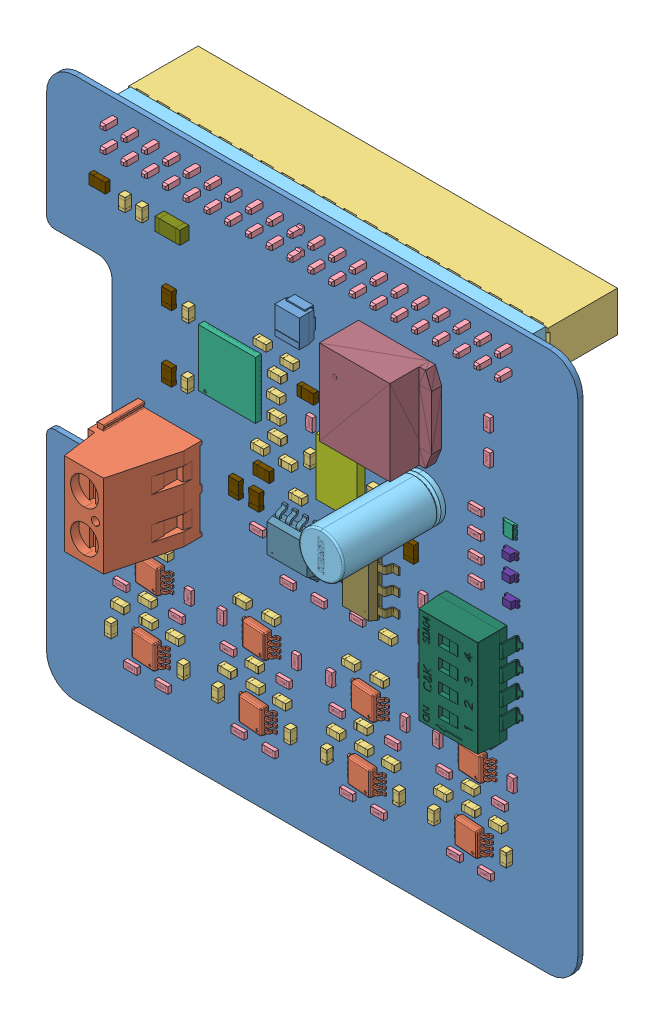
SolidWorks assembly Top, configuration Default. Lengths in mm.
Overall size (64.99 66.2 32.51).
275 component instances, 24 part files, 0 mates.
Components (placement in the parent):
- Top.step-1: Top.step [Default] at origin size (64.99 66.2 32.51)
  - Board.step-1: Board.step [Default] at origin size (64.99 66.2 0.62)
    - Open CASCADE STEP translator 6.8 4.1.1.step-1: Open CASCADE STEP translator 6.8 4.1.1.step [Default] at (0 0 -0.6237) size (64.99 66.2 0.62)
  - U5_amplification3.step-1: U5_amplification3.step [Default] at origin size (4.97 3 1.44)
    - OPA2376AIDGKR--3DModel-STEP-56544.step-1: OPA2376AIDGKR--3DModel-STEP-56544.step [Default] at (49.5292 44.6395 0.3749) x (0 1 0) z (0.997519 0 0.070401) size (3 1.1 4.9)
  - C1_PreAmp3.step-1: C1_PreAmp3.step [Default] at origin size (0.8 1.6 0.8)
    - C0603.step-1: C0603.step [Default] at (53.5531 36.5001 0.4127) x (0 -1 0) z (0 0 1) size (1.6 0.8 0.8)
  - C2_PreAmp3.step-1: C2_PreAmp3.step [Default] at origin size (1.6 0.8 0.8)
    - C0603.step-1: C0603.step [Default] at (45.8499 39.4031 0.4127) x (1 0 0) z (0 0 1) size (1.6 0.8 0.8)
  - C3_PreAmp3.step-1: C3_PreAmp3.step [Default] at origin size (1.6 0.8 0.8)
    - C0603.step-1: C0603.step [Default] at (49.3001 39.4481 0.4127) x (-1 0 0) z (0 0 1) size (1.6 0.8 0.8)
  - C5_PreAmp3.step-1: C5_PreAmp3.step [Default] at origin size (1.6 0.8 0.8)
    - C0603.step-1: C0603.step [Default] at (52.5544 39.4034 0.4127) x (-1 0 0) z (0 0 1) size (1.6 0.8 0.8)
  - C6_PreAmp3.step-1: C6_PreAmp3.step [Default] at origin size (0.8 1.6 0.8)
    - C0603.step-1: C0603.step [Default] at (44.6946 36.5001 0.4127) x (0 -1 0) z (0 0 1) size (1.6 0.8 0.8)
  - C52_amplification3.step-1: C52_amplification3.step [Default] at origin size (1.6 0.8 0.8)
    - C0603.step-1: C0603.step [Default] at (49.2044 41.6576 0.4127) x (-1 0 0) z (0 0 1) size (1.6 0.8 0.8)
  - C54_amplification3.step-1: C54_amplification3.step [Default] at origin size (1.6 0.8 0.8)
    - C0603.step-1: C0603.step [Default] at (47.7041 47.6574 0.4127) x (1 0 0) z (0 0 1) size (1.6 0.8 0.8)
  - C56_amplification3.step-1: C56_amplification3.step [Default] at origin size (1.6 0.8 0.8)
    - C0603.step-1: C0603.step [Default] at (51.2044 47.6576 0.4127) x (-1 0 0) z (0 0 1) size (1.6 0.8 0.8)
  - R1_PreAmp3.step-1: R1_PreAmp3.step [Default] at origin size (0.8 1.6 0.45)
    - R0603.step-1: R0603.step [Default] at (53.5001 36.5001 -0.8615) x (1 0 0) z (0 1 0) size (0.8 0.45 1.6)
  - R2_PreAmp3.step-1: R2_PreAmp3.step [Default] at origin size (1.6 0.8 0.45)
    - R0603.step-1: R0603.step [Default] at (50.9001 33.3448 0.2378) x (0 1 0) z (1 0 0) size (0.8 0.45 1.6)
  - R3_PreAmp3.step-1: R3_PreAmp3.step [Default] at origin size (1.6 0.8 0.45)
    - R0603.step-1: R0603.step [Default] at (47.0999 33.4447 0.2378) x (0 -1 0) z (-1 0 0) size (0.8 0.45 1.6)
  - R4_PreAmp3.step-1: R4_PreAmp3.step [Default] at origin size (0.8 1.6 0.45)
    - R0603.step-1: R0603.step [Default] at (44.6554 36.5044 -0.8615) x (1 0 0) z (0 1 0) size (0.8 0.45 1.6)
  - R23_amplification3.step-1: R23_amplification3.step [Default] at origin size (0.8 1.6 0.45)
    - R0603.step-1: R0603.step [Default] at (54.1042 44.4619 0.2378) x (-1 0 0) z (0 1 0) size (0.8 0.45 1.6)
  - R26_amplification3.step-1: R26_amplification3.step [Default] at origin size (1.6 0.8 0.45)
    - R0603.step-1: R0603.step [Default] at (52.6041 41.5574 0.2378) x (0 -1 0) z (-1 0 0) size (0.8 0.45 1.6)
  - R28_amplification3.step-1: R28_amplification3.step [Default] at origin size (1.6 0.8 0.45)
    - R0603.step-1: R0603.step [Default] at (45.8044 41.5576 0.2378) x (0 1 0) z (1 0 0) size (0.8 0.45 1.6)
  - R38_amplification3.step-1: R38_amplification3.step [Default] at origin size (0.8 1.6 0.45)
    - R0603.step-1: R0603.step [Default] at (44.9999 44.6576 0.2378) x (-1 0 0) z (0 1 0) size (0.8 0.45 1.6)
  - U1_PreAmp3.step-1: U1_PreAmp3.step [Default] at origin size (4.97 3 1.44)
    - OPA2376AIDGKR--3DModel-STEP-56544.step-1: OPA2376AIDGKR--3DModel-STEP-56544.step [Default] at (49.1239 36.474 0.3749) x (0 1 0) z (0.997519 0 0.070401) size (3 1.1 4.9)
  - U5_amplification2.step-1: U5_amplification2.step [Default] at origin size (4.97 3 1.44)
    - OPA2376AIDGKR--3DModel-STEP-56544.step-1: OPA2376AIDGKR--3DModel-STEP-56544.step [Default] at (36.2292 44.5395 0.3749) x (0 1 0) z (0.997519 0 0.070401) size (3 1.1 4.9)
  - C1_PreAmp2.step-1: C1_PreAmp2.step [Default] at origin size (0.8 1.6 0.8)
    - C0603.step-1: C0603.step [Default] at (40.2531 36.4001 0.4127) x (0 -1 0) z (0 0 1) size (1.6 0.8 0.8)
  - C2_PreAmp2.step-1: C2_PreAmp2.step [Default] at origin size (1.6 0.8 0.8)
    - C0603.step-1: C0603.step [Default] at (32.5499 39.3031 0.4127) x (1 0 0) z (0 0 1) size (1.6 0.8 0.8)
  - C3_PreAmp2.step-1: C3_PreAmp2.step [Default] at origin size (1.6 0.8 0.8)
    - C0603.step-1: C0603.step [Default] at (36.0001 39.3481 0.4127) x (-1 0 0) z (0 0 1) size (1.6 0.8 0.8)
  - C5_PreAmp2.step-1: C5_PreAmp2.step [Default] at origin size (1.6 0.8 0.8)
    - C0603.step-1: C0603.step [Default] at (39.2544 39.3034 0.4127) x (-1 0 0) z (0 0 1) size (1.6 0.8 0.8)
  - C6_PreAmp2.step-1: C6_PreAmp2.step [Default] at origin size (0.8 1.6 0.8)
    - C0603.step-1: C0603.step [Default] at (31.3946 36.4001 0.4127) x (0 -1 0) z (0 0 1) size (1.6 0.8 0.8)
  - C52_amplification2.step-1: C52_amplification2.step [Default] at origin size (1.6 0.8 0.8)
    - C0603.step-1: C0603.step [Default] at (35.9044 41.5576 0.4127) x (-1 0 0) z (0 0 1) size (1.6 0.8 0.8)
  - C54_amplification2.step-1: C54_amplification2.step [Default] at origin size (1.6 0.8 0.8)
    - C0603.step-1: C0603.step [Default] at (34.4041 47.5574 0.4127) x (1 0 0) z (0 0 1) size (1.6 0.8 0.8)
  - C56_amplification2.step-1: C56_amplification2.step [Default] at origin size (1.6 0.8 0.8)
    - C0603.step-1: C0603.step [Default] at (37.9044 47.5576 0.4127) x (-1 0 0) z (0 0 1) size (1.6 0.8 0.8)
  - R1_PreAmp2.step-1: R1_PreAmp2.step [Default] at origin size (0.8 1.6 0.45)
    - R0603.step-1: R0603.step [Default] at (40.2001 36.4001 -0.8615) x (1 0 0) z (0 1 0) size (0.8 0.45 1.6)
  - R2_PreAmp2.step-1: R2_PreAmp2.step [Default] at origin size (1.6 0.8 0.45)
    - R0603.step-1: R0603.step [Default] at (37.6001 33.2448 0.2378) x (0 1 0) z (1 0 0) size (0.8 0.45 1.6)
  - R3_PreAmp2.step-1: R3_PreAmp2.step [Default] at origin size (1.6 0.8 0.45)
    - R0603.step-1: R0603.step [Default] at (33.7999 33.3447 0.2378) x (0 -1 0) z (-1 0 0) size (0.8 0.45 1.6)
  - R4_PreAmp2.step-1: R4_PreAmp2.step [Default] at origin size (0.8 1.6 0.45)
    - R0603.step-1: R0603.step [Default] at (31.3553 36.4044 -0.8615) x (1 0 0) z (0 1 0) size (0.8 0.45 1.6)
  - R23_amplification2.step-1: R23_amplification2.step [Default] at origin size (0.8 1.6 0.45)
    - R0603.step-1: R0603.step [Default] at (40.8042 44.3619 0.2378) x (-1 0 0) z (0 1 0) size (0.8 0.45 1.6)
  - R26_amplification2.step-1: R26_amplification2.step [Default] at origin size (1.6 0.8 0.45)
    - R0603.step-1: R0603.step [Default] at (39.3041 41.4574 0.2378) x (0 -1 0) z (-1 0 0) size (0.8 0.45 1.6)
  - R28_amplification2.step-1: R28_amplification2.step [Default] at origin size (1.6 0.8 0.45)
    - R0603.step-1: R0603.step [Default] at (32.5044 41.4576 0.2378) x (0 1 0) z (1 0 0) size (0.8 0.45 1.6)
  - R38_amplification2.step-1: R38_amplification2.step [Default] at origin size (0.8 1.6 0.45)
    - R0603.step-1: R0603.step [Default] at (31.6999 44.5576 0.2378) x (-1 0 0) z (0 1 0) size (0.8 0.45 1.6)
  - U1_PreAmp2.step-1: U1_PreAmp2.step [Default] at origin size (4.97 3 1.44)
    - OPA2376AIDGKR--3DModel-STEP-56544.step-1: OPA2376AIDGKR--3DModel-STEP-56544.step [Default] at (35.8239 36.374 0.3749) x (0 1 0) z (0.997519 0 0.070401) size (3 1.1 4.9)
  - U5_amplification1.step-1: U5_amplification1.step [Default] at origin size (4.97 3 1.44)
    - OPA2376AIDGKR--3DModel-STEP-56544.step-1: OPA2376AIDGKR--3DModel-STEP-56544.step [Default] at (23.1292 44.8395 0.3749) x (0 1 0) z (0.997519 0 0.070401) size (3 1.1 4.9)
  - C1_PreAmp1.step-1: C1_PreAmp1.step [Default] at origin size (0.8 1.6 0.8)
    - C0603.step-1: C0603.step [Default] at (27.1531 36.7001 0.4127) x (0 -1 0) z (0 0 1) size (1.6 0.8 0.8)
  - C2_PreAmp1.step-1: C2_PreAmp1.step [Default] at origin size (1.6 0.8 0.8)
    - C0603.step-1: C0603.step [Default] at (19.4499 39.6032 0.4127) x (1 0 0) z (0 0 1) size (1.6 0.8 0.8)
  - C3_PreAmp1.step-1: C3_PreAmp1.step [Default] at origin size (1.6 0.8 0.8)
    - C0603.step-1: C0603.step [Default] at (22.9001 39.6481 0.4127) x (-1 0 0) z (0 0 1) size (1.6 0.8 0.8)
  - C5_PreAmp1.step-1: C5_PreAmp1.step [Default] at origin size (1.6 0.8 0.8)
    - C0603.step-1: C0603.step [Default] at (26.1544 39.6034 0.4127) x (-1 0 0) z (0 0 1) size (1.6 0.8 0.8)
  - C6_PreAmp1.step-1: C6_PreAmp1.step [Default] at origin size (0.8 1.6 0.8)
    - C0603.step-1: C0603.step [Default] at (18.2946 36.7001 0.4127) x (0 -1 0) z (0 0 1) size (1.6 0.8 0.8)
  - C52_amplification1.step-1: C52_amplification1.step [Default] at origin size (1.6 0.8 0.8)
    - C0603.step-1: C0603.step [Default] at (22.8044 41.8576 0.4127) x (-1 0 0) z (0 0 1) size (1.6 0.8 0.8)
  - C54_amplification1.step-1: C54_amplification1.step [Default] at origin size (1.6 0.8 0.8)
    - C0603.step-1: C0603.step [Default] at (21.3041 47.8574 0.4127) x (1 0 0) z (0 0 1) size (1.6 0.8 0.8)
  - C56_amplification1.step-1: C56_amplification1.step [Default] at origin size (1.6 0.8 0.8)
    - C0603.step-1: C0603.step [Default] at (24.8044 47.8576 0.4127) x (-1 0 0) z (0 0 1) size (1.6 0.8 0.8)
  - R1_PreAmp1.step-1: R1_PreAmp1.step [Default] at origin size (0.8 1.6 0.45)
    - R0603.step-1: R0603.step [Default] at (27.1001 36.7001 -0.8615) x (1 0 0) z (0 1 0) size (0.8 0.45 1.6)
  - R2_PreAmp1.step-1: R2_PreAmp1.step [Default] at origin size (1.6 0.8 0.45)
    - R0603.step-1: R0603.step [Default] at (24.5001 33.5449 0.2378) x (0 1 0) z (1 0 0) size (0.8 0.45 1.6)
  - R3_PreAmp1.step-1: R3_PreAmp1.step [Default] at origin size (1.6 0.8 0.45)
    - R0603.step-1: R0603.step [Default] at (20.6999 33.6447 0.2378) x (0 -1 0) z (-1 0 0) size (0.8 0.45 1.6)
  - R4_PreAmp1.step-1: R4_PreAmp1.step [Default] at origin size (0.8 1.6 0.45)
    - R0603.step-1: R0603.step [Default] at (18.2553 36.7044 -0.8615) x (1 0 0) z (0 1 0) size (0.8 0.45 1.6)
  - R23_amplification1.step-1: R23_amplification1.step [Default] at origin size (0.8 1.6 0.45)
    - R0603.step-1: R0603.step [Default] at (27.7042 44.6619 0.2378) x (-1 0 0) z (0 1 0) size (0.8 0.45 1.6)
  - R26_amplification1.step-1: R26_amplification1.step [Default] at origin size (1.6 0.8 0.45)
    - R0603.step-1: R0603.step [Default] at (26.2041 41.7574 0.2378) x (0 -1 0) z (-1 0 0) size (0.8 0.45 1.6)
  - R28_amplification1.step-1: R28_amplification1.step [Default] at origin size (1.6 0.8 0.45)
    - R0603.step-1: R0603.step [Default] at (19.4044 41.7576 0.2378) x (0 1 0) z (1 0 0) size (0.8 0.45 1.6)
  - R38_amplification1.step-1: R38_amplification1.step [Default] at origin size (0.8 1.6 0.45)
    - R0603.step-1: R0603.step [Default] at (18.5999 44.8576 0.2378) x (-1 0 0) z (0 1 0) size (0.8 0.45 1.6)
  - U1_PreAmp1.step-1: U1_PreAmp1.step [Default] at origin size (4.97 3 1.44)
    - OPA2376AIDGKR--3DModel-STEP-56544.step-1: OPA2376AIDGKR--3DModel-STEP-56544.step [Default] at (22.7239 36.674 0.3749) x (0 1 0) z (0.997519 0 0.070401) size (3 1.1 4.9)
  - R34.step-1: R34.step [Default] at origin size (0.8 1.6 0.45)
    - R0603.step-1: R0603.step [Default] at (56.2999 51.0001 0.2378) x (-1 0 0) z (0 1 0) size (0.8 0.45 1.6)
  - R32.step-1: R32.step [Default] at origin size (0.8 1.6 0.45)
    - R0603.step-1: R0603.step [Default] at (56.2999 58.5001 0.2378) x (-1 0 0) z (0 1 0) size (0.8 0.45 1.6)
  - C7.step-1: C7.step [Default] at origin size (5.5 5.52 32.51)
    - ESK106M035AC3AA.step-1: ESK106M035AC3AA.step [Default] at (56.1001 69.3001 12.5139) x (0 0.000489 -1) z (0 1 0.000489) size (32.51 5.5 5.5)
  - D3.step-1: D3.step [Default] at origin size (1.6 1.6 0.35)
    - LTST-C19HE1WT--3DModel-STEP-56544.step-1: LTST-C19HE1WT--3DModel-STEP-56544.step [Default] at (66.8249 71.2751 0.0128) x (-1 0 0) z (0 1 0) size (1.6 0.35 1.6)
  - XTAL1.step-1: XTAL1.step [Default] at origin size (5 7.52 1.1)
    - 407F35E012M5000.step-1: 407F35E012M5000.step [Default] at (46.5659 66.7521 0.0127) x (0 1 0) z (0 0 1) size (7.52 5 1.1)
      - Body.step-1: Body.step [Default] at (0 0 0.1) size (7 5 1)
      - ('pin.step-1: ('pin.step [Default] at (-3.46 -1.83 0) size (1.72 1.12 0.1)
      - ('pin-0.step-1: ('pin-0.step [Default] at (2.34 -1.83 0) size (1.72 1.12 0.1)
      - ('pin-1.step-1: ('pin-1.step [Default] at (2.34 0.71 0) size (1.72 1.12 0.1)
      - ('pin-2.step-1: ('pin-2.step [Default] at (-3.46 0.71 0) size (1.72 1.12 0.1)
  - U6.step-1: U6.step [Default] at origin size (7.29 6.72 1.81)
    - SOT-223.step-1: SOT-223.step [Default] at (49.5999 57.6675 0.0127) x (0 1 0) z (0 0 1) size (6.72 7.29 1.81)
  - U4.step-1: U4.step [Default] at origin size (12.15 10.61 4.93)
    - TS3B.step-1: TS3B.step [Default] at (53.2512 78.7999 0) x (0 -1 0) z (0 0 1) size (10.61 12.15 4.93)
  - U3.step-1: U3.step [Default] at origin size (5.02 6.2 1.76)
    - D8.step-1: D8.step [Default] at (41.2001 57.0999 0.0127) x (0 1 0) z (0 0 1) size (6.2 5.02 1.76)
  - U1_PreAmp4.step-1: U1_PreAmp4.step [Default] at origin size (4.97 3 1.44)
    - OPA2376AIDGKR--3DModel-STEP-56544.step-1: OPA2376AIDGKR--3DModel-STEP-56544.step [Default] at (62.2239 36.574 0.3749) x (0 1 0) z (0.997519 0 0.070401) size (3 1.1 4.9)
  - S1.step-1: S1.step [Default] at origin size (9.3 12.09 4.5)
    - SDA04H0SBR.step-1: SDA04H0SBR.step [Default] at (63.65 49.6749 2.7626) x (1 0 0) z (0 -1 0) size (9.3 4.5 12.09)
  - R38_amplification4.step-1: R38_amplification4.step [Default] at origin size (0.8 1.6 0.45)
    - R0603.step-1: R0603.step [Default] at (58.0999 44.7576 0.2378) x (-1 0 0) z (0 1 0) size (0.8 0.45 1.6)
  - R37.step-1: R37.step [Default] at origin size (0.8 1.6 0.45)
    - R0603.step-1: R0603.step [Default] at (42.5658 70.4521 0.2378) x (-1 0 0) z (0 1 0) size (0.8 0.45 1.6)
  - R36.step-1: R36.step [Default] at origin size (1.6 0.8 0.45)
    - R0603.step-1: R0603.step [Default] at (48.3001 52.5399 0.2378) x (0 1 0) z (1 0 0) size (0.8 0.45 1.6)
  - R35.step-1: R35.step [Default] at origin size (0.8 1.6 0.45)
    - R0603.step-1: R0603.step [Default] at (56.3001 54.5999 0.2378) x (1 0 0) z (0 -1 0) size (0.8 0.45 1.6)
  - R33.step-1: R33.step [Default] at origin size (1.6 0.8 0.45)
    - R0603.step-1: R0603.step [Default] at (62.8186 66.3499 0.2378) x (0 -1 0) z (-1 0 0) size (0.8 0.45 1.6)
  - R31.step-1: R31.step [Default] at origin size (1.6 0.8 0.45)
    - R0603.step-1: R0603.step [Default] at (62.8189 71.4501 0.2378) x (0 1 0) z (1 0 0) size (0.8 0.45 1.6)
  - R30.step-1: R30.step [Default] at origin size (1.6 0.8 0.45)
    - R0603.step-1: R0603.step [Default] at (62.8186 63.7499 0.2378) x (0 -1 0) z (-1 0 0) size (0.8 0.45 1.6)
  - R29.step-1: R29.step [Default] at origin size (1.6 0.8 0.45)
    - R0603.step-1: R0603.step [Default] at (62.7686 68.8499 0.2378) x (0 -1 0) z (-1 0 0) size (0.8 0.45 1.6)
  - R28_amplification4.step-1: R28_amplification4.step [Default] at origin size (1.6 0.8 0.45)
    - R0603.step-1: R0603.step [Default] at (58.9044 41.6576 0.2378) x (0 1 0) z (1 0 0) size (0.8 0.45 1.6)
  - R27.step-1: R27.step [Default] at origin size (1.6 0.8 0.45)
    - R0603.step-1: R0603.step [Default] at (36.0999 55.8999 0.2378) x (0 -1 0) z (-1 0 0) size (0.8 0.45 1.6)
  - R26_amplification4.step-1: R26_amplification4.step [Default] at origin size (1.6 0.8 0.45)
    - R0603.step-1: R0603.step [Default] at (65.7041 41.6574 0.2378) x (0 -1 0) z (-1 0 0) size (0.8 0.45 1.6)
  - R23_amplification4.step-1: R23_amplification4.step [Default] at origin size (0.8 1.6 0.45)
    - R0603.step-1: R0603.step [Default] at (67.2042 44.5619 0.2378) x (-1 0 0) z (0 1 0) size (0.8 0.45 1.6)
  - R22.step-1: R22.step [Default] at origin size (1.6 0.8 0.45)
    - R0603.step-1: R0603.step [Default] at (43.5999 52.1107 0.2378) x (0 -1 0) z (-1 0 0) size (0.8 0.45 1.6)
  - R21.step-1: R21.step [Default] at origin size (1.6 0.8 0.45)
    - R0603.step-1: R0603.step [Default] at (39.8001 52.1108 0.2378) x (0 1 0) z (1 0 0) size (0.8 0.45 1.6)
  - R20.step-1: R20.step [Default] at origin size (0.8 1.6 0.45)
    - R0603.step-1: R0603.step [Default] at (64.3001 81.2999 0.2378) x (1 0 0) z (0 -1 0) size (0.8 0.45 1.6)
  - R19.step-1: R19.step [Default] at origin size (0.8 1.6 0.45)
    - R0603.step-1: R0603.step [Default] at (64.3001 77.5999 0.2378) x (1 0 0) z (0 -1 0) size (0.8 0.45 1.6)
  - R18.step-1: R18.step [Default] at origin size (1.6 0.8 0.45)
    - R0603.step-1: R0603.step [Default] at (39.966 64.9519 -0.8615) x (0 -1 0) z (1 0 0) size (0.8 0.45 1.6)
  - R17.step-1: R17.step [Default] at origin size (1.6 0.8 0.45)
    - R0603.step-1: R0603.step [Default] at (30.1001 76.3999 -0.8615) x (0 -1 0) z (1 0 0) size (0.8 0.45 1.6)
  - R4_PreAmp4.step-1: R4_PreAmp4.step [Default] at origin size (0.8 1.6 0.45)
    - R0603.step-1: R0603.step [Default] at (57.7553 36.6044 -0.8615) x (1 0 0) z (0 1 0) size (0.8 0.45 1.6)
  - R3_PreAmp4.step-1: R3_PreAmp4.step [Default] at origin size (1.6 0.8 0.45)
    - R0603.step-1: R0603.step [Default] at (60.1999 33.5447 0.2378) x (0 -1 0) z (-1 0 0) size (0.8 0.45 1.6)
  - R2_PreAmp4.step-1: R2_PreAmp4.step [Default] at origin size (1.6 0.8 0.45)
    - R0603.step-1: R0603.step [Default] at (64.0001 33.4448 0.2378) x (0 1 0) z (1 0 0) size (0.8 0.45 1.6)
  - R1_PreAmp4.step-1: R1_PreAmp4.step [Default] at origin size (0.8 1.6 0.45)
    - R0603.step-1: R0603.step [Default] at (66.6001 36.6001 -0.8615) x (1 0 0) z (0 1 0) size (0.8 0.45 1.6)
  - F1.step-1: F1.step [Default] at origin size (3.02 1.63 1.13)
    - F1206.step-1: F1206.step [Default] at (25.9001 82.9 0.0138) x (-1 0 0) z (0 1 0) size (3.02 1.13 1.63)
  - D4.step-1: D4.step [Default] at origin size (1.6 0.8 0.8)
    - LTST-C190KRKT--3DModel-STEP-56544.step-1: LTST-C190KRKT--3DModel-STEP-56544.step [Default] at (67.0189 66.5501 0.0128) x (0 1 0) z (1 0 0) size (0.8 0.8 1.6)
  - D2.step-1: D2.step [Default] at origin size (1.6 0.8 0.8)
    - LTST-C190KRKT--3DModel-STEP-56544.step-1: LTST-C190KRKT--3DModel-STEP-56544.step [Default] at (67.1189 63.8501 0.0128) x (0 1 0) z (1 0 0) size (0.8 0.8 1.6)
  - D1.step-1: D1.step [Default] at origin size (1.6 0.8 0.8)
    - LTST-C190KRKT--3DModel-STEP-56544.step-1: LTST-C190KRKT--3DModel-STEP-56544.step [Default] at (67.0189 68.8501 0.0128) x (0 1 0) z (1 0 0) size (0.8 0.8 1.6)
  - C56_amplification4.step-1: C56_amplification4.step [Default] at origin size (1.6 0.8 0.8)
    - C0603.step-1: C0603.step [Default] at (64.3044 47.7576 0.4127) x (-1 0 0) z (0 0 1) size (1.6 0.8 0.8)
  - C54_amplification4.step-1: C54_amplification4.step [Default] at origin size (1.6 0.8 0.8)
    - C0603.step-1: C0603.step [Default] at (60.8041 47.7574 0.4127) x (1 0 0) z (0 0 1) size (1.6 0.8 0.8)
  - C52_amplification4.step-1: C52_amplification4.step [Default] at origin size (1.6 0.8 0.8)
    - C0603.step-1: C0603.step [Default] at (62.3044 41.7576 0.4127) x (-1 0 0) z (0 0 1) size (1.6 0.8 0.8)
  - C50.step-1: C50.step [Default] at origin size (0.8 1.6 0.8)
    - C0603.step-1: C0603.step [Default] at (42.6658 66.8021 0.4127) x (0 -1 0) z (0 0 1) size (1.6 0.8 0.8)
  - C49.step-1: C49.step [Default] at origin size (0.8 1.6 0.8)
    - C0603.step-1: C0603.step [Default] at (50.366 67.0519 0.4127) x (0 1 0) z (0 0 1) size (1.6 0.8 0.8)
  - C48.step-1: C48.step [Default] at origin size (1.6 0.8 0.8)
    - C0603.step-1: C0603.step [Default] at (52.1999 52.6397 0.4127) x (1 0 0) z (0 0 1) size (1.6 0.8 0.8)
  - C47.step-1: C47.step [Default] at origin size (0.8 1.6 0.8)
    - C0603.step-1: C0603.step [Default] at (20.0001 82.6999 0.4127) x (0 1 0) z (0 0 1) size (1.6 0.8 0.8)
  - C46.step-1: C46.step [Default] at origin size (0.8 1.6 0.8)
    - C0603.step-1: C0603.step [Default] at (22.1001 82.6499 0.4127) x (0 1 0) z (0 0 1) size (1.6 0.8 0.8)
  - C45.step-1: C45.step [Default] at origin size (2 1.25 0.6)
    - C0805.step-1: C0805.step [Default] at (16.7999 83.0999 0.3128) x (1 0 0) z (0 -1 0) size (2 0.6 1.25)
  - C44.step-1: C44.step [Default] at origin size (1.6 0.8 0.8)
    - C0603.step-1: C0603.step [Default] at (36.0999 55.9001 -1.0364) x (1 0 0) z (0 0 -1) size (1.6 0.8 0.8)
  - C43.step-1: C43.step [Default] at origin size (1.6 0.8 0.8)
    - C0603.step-1: C0603.step [Default] at (41.2001 61.9894 0.4127) x (-1 0 0) z (0 0 1) size (1.6 0.8 0.8)
  - C42.step-1: C42.step [Default] at origin size (3.02 3.68 2.13)
    - CAP_3_5X2_8X1_9.step-1: CAP_3_5X2_8X1_9.step [Default] at (41.5001 80.9999 0) x (0 1 0) z (0 0 1) size (3.68 3.02 2.13)
  - C39.step-1: C39.step [Default] at origin size (1.25 2 0.6)
    - C0805.step-1: C0805.step [Default] at (54.9001 63.0999 0.3128) x (0 1 0) z (1 0 0) size (2 0.6 1.25)
  - C38.step-1: C38.step [Default] at origin size (1.6 0.8 0.8)
    - C0603.step-1: C0603.step [Default] at (38.6658 67.0519 0.4127) x (1 0 0) z (0 0 1) size (1.6 0.8 0.8)
  - C37.step-1: C37.step [Default] at origin size (1.6 0.8 0.8)
    - C0603.step-1: C0603.step [Default] at (38.5658 69.1519 0.4127) x (1 0 0) z (0 0 1) size (1.6 0.8 0.8)
  - C36.step-1: C36.step [Default] at origin size (2 1.25 0.6)
    - C0805.step-1: C0805.step [Default] at (38.5658 69.1521 -0.9365) x (1 0 0) z (0 1 0) size (2 0.6 1.25)
  - C35.step-1: C35.step [Default] at origin size (1.6 0.8 0.8)
    - C0603.step-1: C0603.step [Default] at (39.9658 64.9519 0.4127) x (1 0 0) z (0 0 1) size (1.6 0.8 0.8)
  - C34.step-1: C34.step [Default] at origin size (1.6 0.8 0.8)
    - C0603.step-1: C0603.step [Default] at (40.1658 75.7519 0.4127) x (1 0 0) z (0 0 1) size (1.6 0.8 0.8)
  - C33.step-1: C33.step [Default] at origin size (1.6 0.8 0.8)
    - C0603.step-1: C0603.step [Default] at (38.6658 73.6519 0.4127) x (1 0 0) z (0 0 1) size (1.6 0.8 0.8)
  - C32.step-1: C32.step [Default] at origin size (2 1.25 0.6)
    - C0805.step-1: C0805.step [Default] at (42.2658 73.4519 0.3128) x (1 0 0) z (0 -1 0) size (2 0.6 1.25)
  - C31.step-1: C31.step [Default] at origin size (1.25 2 0.6)
    - C0805.step-1: C0805.step [Default] at (33.466 59.1519 0.3128) x (0 1 0) z (1 0 0) size (2 0.6 1.25)
  - C30.step-1: C30.step [Default] at origin size (0.8 1.6 0.8)
    - C0603.step-1: C0603.step [Default] at (27.666 67.3519 0.4127) x (0 1 0) z (0 0 1) size (1.6 0.8 0.8)
  - C29.step-1: C29.step [Default] at origin size (1.25 2 0.6)
    - C0805.step-1: C0805.step [Default] at (25.2659 67.0521 0.3128) x (0 -1 0) z (-1 0 0) size (2 0.6 1.25)
  - C28.step-1: C28.step [Default] at origin size (1.6 0.8 0.8)
    - C0603.step-1: C0603.step [Default] at (38.516 71.3521 0.4127) x (-1 0 0) z (0 0 1) size (1.6 0.8 0.8)
  - C27.step-1: C27.step [Default] at origin size (2 1.25 0.6)
    - C0805.step-1: C0805.step [Default] at (38.5658 71.7521 -0.9365) x (1 0 0) z (0 1 0) size (2 0.6 1.25)
  - C26.step-1: C26.step [Default] at origin size (1.6 0.8 0.8)
    - C0603.step-1: C0603.step [Default] at (36.566 64.9521 0.4127) x (-1 0 0) z (0 0 1) size (1.6 0.8 0.8)
  - C25.step-1: C25.step [Default] at origin size (2 1.25 0.6)
    - C0805.step-1: C0805.step [Default] at (36.8616 62.4519 0.3128) x (1 0 0) z (0 -1 0) size (2 0.6 1.25)
  - C24.step-1: C24.step [Default] at origin size (1.25 2 0.6)
    - C0805.step-1: C0805.step [Default] at (35.966 59.1519 0.3128) x (0 1 0) z (1 0 0) size (2 0.6 1.25)
  - C23.step-1: C23.step [Default] at origin size (1.6 0.8 0.8)
    - C0603.step-1: C0603.step [Default] at (36.8658 76.1519 0.4127) x (1 0 0) z (0 0 1) size (1.6 0.8 0.8)
  - C22.step-1: C22.step [Default] at origin size (2 1.25 0.6)
    - C0805.step-1: C0805.step [Default] at (36.816 76.1519 -0.9365) x (-1 0 0) z (0 -1 0) size (2 0.6 1.25)
  - C21.step-1: C21.step [Default] at origin size (0.8 1.6 0.8)
    - C0603.step-1: C0603.step [Default] at (27.766 74.8519 0.4127) x (0 1 0) z (0 0 1) size (1.6 0.8 0.8)
  - C20.step-1: C20.step [Default] at origin size (1.25 2 0.6)
    - C0805.step-1: C0805.step [Default] at (25.2659 75.1521 0.3128) x (0 -1 0) z (-1 0 0) size (2 0.6 1.25)
  - C6_PreAmp4.step-1: C6_PreAmp4.step [Default] at origin size (0.8 1.6 0.8)
    - C0603.step-1: C0603.step [Default] at (57.7946 36.6001 0.4127) x (0 -1 0) z (0 0 1) size (1.6 0.8 0.8)
  - C5_PreAmp4.step-1: C5_PreAmp4.step [Default] at origin size (1.6 0.8 0.8)
    - C0603.step-1: C0603.step [Default] at (65.6544 39.5034 0.4127) x (-1 0 0) z (0 0 1) size (1.6 0.8 0.8)
  - C4.step-1: C4.step [Default] at origin size (0.8 1.6 0.8)
    - C0603.step-1: C0603.step [Default] at (50.7999 63.4001 0.4127) x (0 -1 0) z (0 0 1) size (1.6 0.8 0.8)
  - C3_PreAmp4.step-1: C3_PreAmp4.step [Default] at origin size (1.6 0.8 0.8)
    - C0603.step-1: C0603.step [Default] at (62.4001 39.5481 0.4127) x (-1 0 0) z (0 0 1) size (1.6 0.8 0.8)
  - C2_PreAmp4.step-1: C2_PreAmp4.step [Default] at origin size (1.6 0.8 0.8)
    - C0603.step-1: C0603.step [Default] at (58.9499 39.5031 0.4127) x (1 0 0) z (0 0 1) size (1.6 0.8 0.8)
  - C1_PreAmp4.step-1: C1_PreAmp4.step [Default] at origin size (0.8 1.6 0.8)
    - C0603.step-1: C0603.step [Default] at (66.6531 36.6001 0.4127) x (0 -1 0) z (0 0 1) size (1.6 0.8 0.8)
  - B1.step-1: B1.step [Default] at origin size (8.2 10.76 13.5)
    - c-282837-2-g2-3d.step-1: c-282837-2-g2-3d.step [Default] at (20.7999 56.6001 2.7628) x (0 -1 0) z (-1 0 0) size (10.76 13.5 8.2)
  - U5_amplification4.step-1: U5_amplification4.step [Default] at origin size (4.97 3 1.44)
    - OPA2376AIDGKR--3DModel-STEP-56544.step-1: OPA2376AIDGKR--3DModel-STEP-56544.step [Default] at (62.6292 44.7395 0.3749) x (0 1 0) z (0.997519 0 0.070401) size (3 1.1 4.9)
  - J3.step-1: J3.step [Default] at origin size (51.31 5.08 13.34)
    - ESQ-120-12-G-D-LL.step-1: ESQ-120-12-G-D-LL.step [Default] at (42.5019 89.0799 -3.1765) x (-1 0 0) z (0 -1 0) size (51.31 13.33 5.08)
      - _ESQ-120-12-G-D-LL_socket.step-1: _ESQ-120-12-G-D-LL_socket.step [Default] at (-25.654 0 0) size (51.31 8.51 4.95)
      - _ESQ-120-12-G-D-LL_pins.step-1: _ESQ-120-12-G-D-LL_pins.step [Default] at origin size (50.55 9.77 4.7)
      - _ESQ-120-12-G-D-LL_bpins.step-1: _ESQ-120-12-G-D-LL_bpins.step [Default] at (-25.527 -2.54 0) size (50.8 2.54 5.08)
  - U2.step-1: U2.step [Default] at origin size (7 7 0.73)
    - ADI-CS-48-1.step-1: ADI-CS-48-1.step [Default] at (32.8659 71.052 0) x (0 1 0) z (0 0 1) size (7 7 0.73)
